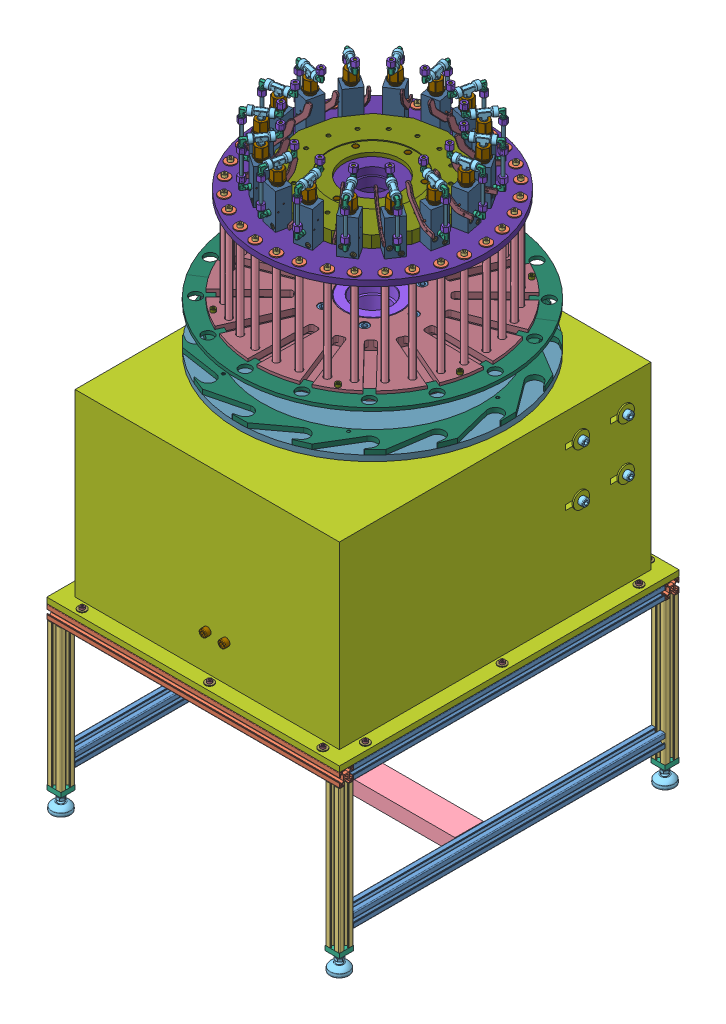
SolidWorks assembly Assieme_FINALE, configuration Default. Lengths in mm.
Overall size (1084.72 1264.83 1084.72).
659 component instances, 53 part files, 36 mates.
Components (placement in the parent):
- SupportoBase_Totale-2: SupportoBase_Totale [Default] at (4.0127 -14.4529 -3.9361) x (0 1 0) z (0 0 1) size (801.2 636.12 736.12)
  - Supporto_base_macchina-1: Supporto_base_macchina [Default] at origin size (378.2 636.12 736.12)
    - profilato_30x30_590-3: profilato_30x30_590 [Default] at (275.414 713.7262 -66.645) size (30 30 660)
    - profilato_30x30_590-5: profilato_30x30_590 [Default] at (275.414 123.7262 -66.645) size (30 30 660)
    - profilato_30x30_550-5: profilato_30x30_550 [Default] at (275.414 703.7262 -716.645) x (1 0 0) z (0 1 0) size (30 30 620)
    - profilato_30x30_550-6: profilato_30x30_550 [Default] at (275.414 703.7262 -26.645) x (1 0 0) z (0 1 0) size (30 30 620)
    - profilato_30x30_272-5: profilato_30x30_272 [Default] at (-16.586 123.7262 -716.645) x (0 0 1) z (-1 0 0) size (30 30 302)
    - profilato_30x30_272-6: profilato_30x30_272 [Default] at (-16.586 713.7262 -716.645) x (0 0 1) z (-1 0 0) size (30 30 302)
    - profilato_30x30_272-7: profilato_30x30_272 [Default] at (235.414 123.7262 -26.645) x (0 0 -1) z (1 0 0) size (30 30 302)
    - profilato_30x30_272-8: profilato_30x30_272 [Default] at (-16.586 713.7262 -26.645) x (0 0 1) z (-1 0 0) size (30 30 302)
    - profilo_U_60x30_490_supporto_base_macchina-1: profilo_U_60x30_490_supporto_base_macchina [Default] at (15.1 707.7262 -323.6583) x (0 0 1) z (0 -1 0) size (60 30 569)
    - profilato_30x30_590-6: profilato_30x30_590 [Default] at (3.414 123.7262 -66.645) size (30 30 660)
    - profilato_30x30_590-7: profilato_30x30_590 [Default] at (3.414 713.7262 -676.645) x (-1 0 0) z (0 0 -1) size (30 30 660)
    - 6322125-1: 6322125 [Default] at (-85.2818 713.7262 -26.645) x (0 0 -1) z (1 0 0) size (40 40 71.2)
    - 6322125-2: 6322125 [Default] at (-85.2818 713.7262 -716.645) x (0 0 -1) z (1 0 0) size (40 40 71.2)
    - 6322125-3: 6322125 [Default] at (-85.2818 123.7262 -26.645) x (0 -0.924225 -0.381849) z (1 0 0) size (40 40 71.2)
    - 6322125-4: 6322125 [Default] at (-85.2818 123.7262 -716.645) x (0 0 -1) z (1 0 0) size (40 40 71.2)
    - tappo_filettato_Supporto_base_macchina-1: tappo_filettato_Supporto_base_macchina [Default] at (-41.586 123.7262 -26.645) x (0 0 1) z (-1 0 0) size (30 30 10.37)
    - tappo_filettato_Supporto_base_macchina-2: tappo_filettato_Supporto_base_macchina [Default] at (-41.586 123.7262 -716.645) x (0 0 1) z (-1 0 0) size (30 30 10.37)
    - tappo_filettato_Supporto_base_macchina-3: tappo_filettato_Supporto_base_macchina [Default] at (-41.586 713.7262 -716.645) x (0 0 1) z (-1 0 0) size (30 30 10.37)
    - tappo_filettato_Supporto_base_macchina-4: tappo_filettato_Supporto_base_macchina [Default] at (-51.586 713.7262 -26.645) x (0 0 -1) z (1 0 0) size (30 30 10.37)
  - assieme_base-1: assieme_base [Default] at (466.8009 1138.7262 -472.0974) x (0 0 -1) z (0 -1 0) size (720 423 620)
    - Supporto di Base per macchina-1: Supporto di Base per macchina [Default] at (-460.4524 -176.3869 1030) size (720 403 620)
    - canotto di supporto-1: canotto di supporto [Default] at (-100.4524 134.8265 740) x (0 1 0) z (-0.866025 0 0.5) size (220 238 238)
    - m10 35mm-7: m10 35mm [ISO 4762 M10 x 35 - 35N] at (4.5476 246.6131 740) x (0 -1 0) z (1 0 0) size (45 16 16)
    - m10 35mm-8: m10 35mm [ISO 4762 M10 x 35 - 35N] at (-47.9524 246.6131 649.0673) x (0 -1 0) z (0.5 0 -0.866025) size (45 16 16)
    - m10 35mm-9: m10 35mm [ISO 4762 M10 x 35 - 35N] at (-152.9524 246.6131 649.0673) x (0 -1 0) z (-0.5 0 -0.866025) size (45 16 16)
    - m10 35mm-10: m10 35mm [ISO 4762 M10 x 35 - 35N] at (-205.4524 246.6131 740) x (0 -1 0) z (-1 0 0) size (45 16 16)
    - m10 35mm-11: m10 35mm [ISO 4762 M10 x 35 - 35N] at (-152.9524 246.6131 830.9327) x (0 -1 0) z (-0.5 0 0.866025) size (45 16 16)
    - m10 35mm-12: m10 35mm [ISO 4762 M10 x 35 - 35N] at (-47.9524 246.6131 830.9327) x (0 -1 0) z (0.5 0 0.866025) size (45 16 16)
    - Traversa di blocco albero-1: Traversa di blocco albero [Default] at (-100.4524 -86.3869 772.5) size (644 42 65)
    - m10 35mm-13: m10 35mm [ISO 4762 M10 x 35 - 35N] at (239.5476 -86.3869 760) x (-1 0 0) z (0 -1 0) size (45 16 16)
    - m10 35mm-16: m10 35mm [ISO 4762 M10 x 35 - 35N] at (239.5476 -86.3869 720) x (-1 0 0) z (0 -1 0) size (45 16 16)
    - m10 35mm-17: m10 35mm [ISO 4762 M10 x 35 - 35N] at (-440.4524 -86.3869 720) x (1 0 0) z (0 1 0) size (45 16 16)
    - m10 35mm-18: m10 35mm [ISO 4762 M10 x 35 - 35N] at (-440.4524 -86.3869 760) x (1 0 0) z (0 1 0) size (45 16 16)
  - DadoT-2: DadoT [Default] at (288.4104 668.7262 -716.645) x (0 0 -1) z (0 -1 0) size (16.5 6 8)
  - DadoT-9: DadoT [Default] at (288.4104 668.7262 -26.645) x (0 0 -1) z (0 -1 0) size (16.5 6 8)
  - DadoT-10: DadoT [Default] at (288.6104 713.7262 -661.645) x (0 1 0) z (0 0 -1) size (16.5 6 8)
  - DadoT-11: DadoT [Default] at (288.6104 713.7262 -371.645) x (0 1 0) z (0 0 -1) size (16.5 6 8)
  - DadoT-12: DadoT [Default] at (288.6104 713.7262 -81.645) x (0 1 0) z (0 0 -1) size (16.5 6 8)
  - DadoT-13: DadoT [Default] at (288.6104 123.7262 -661.645) x (0 1 0) z (0 0 -1) size (16.5 6 8)
  - DadoT-15: DadoT [Default] at (288.6104 123.7262 -371.645) x (0 1 0) z (0 0 -1) size (16.5 6 8)
  - DadoT-17: DadoT [Default] at (288.6104 123.7262 -81.645) x (0 1 0) z (0 0 -1) size (16.5 6 8)
  - RosettaM6-1: RosettaM6 [Washer ISO 7093 - 6] at (302.414 713.7262 -661.645) x (-1 0 0) z (0 0 1) size (1.6 18 18)
  - ViteM6-20-1: ViteM6-20 [ISO 4762 M6 x 20 - 20S] at (308.414 713.7262 -661.645) x (-1 0 0) z (0 0 1) size (26 10 10)
  - RosettaM6-2: RosettaM6 [Washer ISO 7093 - 6] at (302.414 668.7262 -716.645) x (-1 0 0) z (0 0 1) size (1.6 18 18)
  - ViteM6-20-2: ViteM6-20 [ISO 4762 M6 x 20 - 20S] at (308.414 668.7262 -716.645) x (-1 0 0) z (0 0 1) size (26 10 10)
  - RosettaM6-3: RosettaM6 [Washer ISO 7093 - 6] at (302.414 713.7262 -371.645) x (-1 0 0) z (0 0 1) size (1.6 18 18)
  - RosettaM6-4: RosettaM6 [Washer ISO 7093 - 6] at (302.414 713.7262 -81.645) x (-1 0 0) z (0 0 1) size (1.6 18 18)
  - ViteM6-20-3: ViteM6-20 [ISO 4762 M6 x 20 - 20S] at (308.414 713.7262 -371.645) x (-1 0 0) z (0 0 1) size (26 10 10)
  - ViteM6-20-4: ViteM6-20 [ISO 4762 M6 x 20 - 20S] at (308.414 713.7262 -81.645) x (-1 0 0) z (0 0 1) size (26 10 10)
  - RosettaM6-5: RosettaM6 [Washer ISO 7093 - 6] at (302.414 123.7262 -661.645) x (-1 0 0) z (0 0 1) size (1.6 18 18)
  - ViteM6-20-5: ViteM6-20 [ISO 4762 M6 x 20 - 20S] at (308.414 123.7262 -661.645) x (-1 0 0) z (0 0 1) size (26 10 10)
  - RosettaM6-6: RosettaM6 [Washer ISO 7093 - 6] at (302.414 123.7262 -371.645) x (-1 0 0) z (0 0 1) size (1.6 18 18)
  - RosettaM6-7: RosettaM6 [Washer ISO 7093 - 6] at (302.414 123.7262 -81.645) x (-1 0 0) z (0 0 1) size (1.6 18 18)
  - ViteM6-20-6: ViteM6-20 [ISO 4762 M6 x 20 - 20S] at (308.414 123.7262 -371.645) x (-1 0 0) z (0 0 1) size (26 10 10)
  - ViteM6-20-7: ViteM6-20 [ISO 4762 M6 x 20 - 20S] at (308.414 123.7262 -81.645) x (-1 0 0) z (0 0 1) size (26 10 10)
  - ViteM6-20-8: ViteM6-20 [ISO 4762 M6 x 20 - 20S] at (308.414 398.7262 -716.645) x (-1 0 0) z (0 0 1) size (26 10 10)
  - RosettaM6-8: RosettaM6 [Washer ISO 7093 - 6] at (302.414 398.7262 -716.645) x (-1 0 0) z (0 0 1) size (1.6 18 18)
  - DadoT-19: DadoT [Default] at (288.4104 398.7262 -716.645) x (0 0 -1) z (0 -1 0) size (16.5 6 8)
  - DadoT-20: DadoT [Default] at (288.4104 158.7262 -716.645) x (0 0 -1) z (0 -1 0) size (16.5 6 8)
  - RosettaM6-9: RosettaM6 [Washer ISO 7093 - 6] at (302.414 158.7262 -716.645) x (-1 0 0) z (0 0 1) size (1.6 18 18)
  - ViteM6-20-9: ViteM6-20 [ISO 4762 M6 x 20 - 20S] at (308.414 158.7262 -716.645) x (-1 0 0) z (0 0 1) size (26 10 10)
  - DadoT-21: DadoT [Default] at (288.4104 668.7262 -26.645) x (0 0 -1) z (0 -1 0) size (16.5 6 8)
  - RosettaM6-10: RosettaM6 [Washer ISO 7093 - 6] at (302.414 668.7262 -26.645) x (-1 0 0) z (0 0 1) size (1.6 18 18)
  - ViteM6-20-10: ViteM6-20 [ISO 4762 M6 x 20 - 20S] at (308.414 668.7262 -26.645) x (-1 0 0) z (0 0 1) size (26 10 10)
  - DadoT-22: DadoT [Default] at (288.4104 158.7262 -26.645) x (0 0 -1) z (0 -1 0) size (16.5 6 8)
  - RosettaM6-11: RosettaM6 [Washer ISO 7093 - 6] at (302.414 158.7262 -26.645) x (-1 0 0) z (0 0 1) size (1.6 18 18)
  - ViteM6-20-11: ViteM6-20 [ISO 4762 M6 x 20 - 20S] at (308.414 158.7262 -26.645) x (-1 0 0) z (0 0 1) size (26 10 10)
  - ViteM6-20-12: ViteM6-20 [ISO 4762 M6 x 20 - 20S] at (308.414 398.7262 -26.645) x (-1 0 0) z (0 0 1) size (26 10 10)
  - RosettaM6-12: RosettaM6 [Washer ISO 7093 - 6] at (302.414 398.7262 -26.645) x (-1 0 0) z (0 0 1) size (1.6 18 18)
  - DadoT-23: DadoT [Default] at (288.4104 398.7262 -26.645) x (0 0 -1) z (0 -1 0) size (16.5 6 8)
- motoriduttore-1: motoriduttore [Default] at (-164.7135 275.9611 -1179.5811) x (0 0 1) z (-1 0 0) size (200 160 175)
- Assieme_Riduttore-1: Assieme_Riduttore [Default] at (-346.4148 520.923 -401.8673) x (0 1 0) z (0.342115 0 -0.939658) size (226 168.82 169.04)
  - AlberoRiduttore-1: AlberoRiduttore [Default] at (-61.6906 7.4655 211) size (201 29 29)
  - linguetta_uni6604_b_8x7x50-1: linguetta_uni6604_b_8x7x50 [Default] at (-116.7419 7.4655 226) x (1 0 0) z (0 1 0) size (50 7 8)
  - linguetta_uni6604_b_8x7x35-1: linguetta_uni6604_b_8x7x35 [Default] at (-33.7419 7.4655 226.5) x (1 0 0) z (0 1 0) size (35 7 8)
  - linguetta_uni6604_b_8x7x35-2: linguetta_uni6604_b_8x7x35 [Default] at (41.2581 7.4655 226.5) x (1 0 0) z (0 1 0) size (35 7 8)
  - ASSIEME-LASS-90-VERS-B-O-25-3D.step-1: ASSIEME-LASS-90-VERS-B-O-25-3D.step [Default] at (-111.3519 -70.5563 279.3493) x (-1 0 0) z (0 0.707107 -0.707107) size (64.28 105 105)
  - Rondella di fermo-1: Rondella di fermo [Default] at (-122.7419 7.4655 211) x (0 0.707107 -0.707107) z (-1 0 0) size (36 36 3)
  - M8 25 mm-1: M8 25 mm [ISO 4762 M8 x 25 - 25N] at (92.2581 7.4655 211) x (-1 0 0) z (0 1 0) size (33 13 13)
  - M8 25 mm-2: M8 25 mm [ISO 4762 M8 x 25 - 25N] at (-133.7419 7.4655 211) x (1 0 0) z (0 -0.707107 0.707107) size (33 13 13)
  - M6 16mm-3: M6 16mm [ISO 4762 M6 x 16 - 16N] at (-44.8119 40.5589 196.8286) x (-1 0 0) z (0 0.935687 0.352831) size (22 10 10)
  - M6 16mm-14: M6 16mm [ISO 4762 M6 x 16 - 16N] at (-44.8119 11.7394 175.2546) x (-1 0 0) z (0 0.773404 -0.633913) size (22 10 10)
  - M6 16mm-15: M6 16mm [ISO 4762 M6 x 16 - 16N] at (-44.8119 -21.354 189.426) x (-1 0 0) z (0 -0.162283 -0.986744) size (22 10 10)
  - M6 16mm-16: M6 16mm [ISO 4762 M6 x 16 - 16N] at (-44.8119 -25.6279 225.1714) x (-1 0 0) z (0 -0.935687 -0.352831) size (22 10 10)
  - M6 16mm-17: M6 16mm [ISO 4762 M6 x 16 - 16N] at (-44.8119 3.1916 246.7454) x (-1 0 0) z (0 -0.773404 0.633913) size (22 10 10)
  - M6 16mm-18: M6 16mm [ISO 4762 M6 x 16 - 16N] at (-44.8119 36.285 232.574) x (-1 0 0) z (0 0.162283 0.986744) size (22 10 10)
  - Parte1^Assieme_Riduttore-1: Parte1^Assieme_Riduttore [Default] at origin (virtual)
  - ruota dentata m22-4: ruota dentata m22 [Chain wheel ISO - 22Z 10A-1 --22SA36.0N] at (-59.7419 7.4655 211) x (1 0 0) z (0 -0.599278 0.800541) size (8.93 120.13 121.23)
  - Rondella di fermo-2: Rondella di fermo [Default] at (84.2581 7.4655 211) x (0 0 1) z (-1 0 0) size (36 36 3)
- socket head cap screw_iso-1: socket head cap screw_iso [ISO 4762 M10 x 40 - 40N] at (-121.7135 603.4611 -555.5811) x (-1 0 0) z (0 -0.924225 -0.381849) size (50 16 16)
- socket head cap screw_iso-2: socket head cap screw_iso [ISO 4762 M10 x 40 - 40N] at (-121.7135 492.4611 -555.5811) x (-1 0 0) z (0 0 1) size (50 16 16)
- socket head cap screw_iso-3: socket head cap screw_iso [ISO 4762 M10 x 40 - 40N] at (-121.7135 603.4611 -650.5811) x (-1 0 0) z (0 0 1) size (50 16 16)
- socket head cap screw_iso-4: socket head cap screw_iso [ISO 4762 M10 x 40 - 40N] at (-121.7135 492.4611 -650.5811) x (-1 0 0) z (0 0 1) size (50 16 16)
- hex nut style 2 gradeab_iso-1: hex nut style 2 gradeab_iso [ISO - 4033 - M10 - W - N] at (-174.0135 603.4611 -650.5811) x (0 0 1) z (-1 0 0) size (16 18.48 9.3)
- hex nut style 2 gradeab_iso-2: hex nut style 2 gradeab_iso [ISO - 4033 - M10 - W - N] at (-174.0135 603.4611 -555.5811) x (0 0 1) z (-1 0 0) size (16 18.48 9.3)
- hex nut style 2 gradeab_iso-3: hex nut style 2 gradeab_iso [ISO - 4033 - M10 - W - N] at (-174.0135 492.4611 -650.5811) x (0 0 1) z (-1 0 0) size (16 18.48 9.3)
- hex nut style 2 gradeab_iso-4: hex nut style 2 gradeab_iso [ISO - 4033 - M10 - W - N] at (-174.0135 492.4611 -555.5811) x (0 0 1) z (-1 0 0) size (16 18.48 9.3)
- plain washer xlarge grade c_iso-1: plain washer xlarge grade c_iso [Washer ISO 7094 - 10] at (-134.7135 603.4611 -555.5811) x (-1 0 0) z (0 0.924225 0.381849) size (3 34 34)
- plain washer xlarge grade c_iso-2: plain washer xlarge grade c_iso [Washer ISO 7094 - 10] at (-134.7135 492.4611 -555.5811) x (-1 0 0) z (0 0 1) size (3 34 34)
- plain washer xlarge grade c_iso-3: plain washer xlarge grade c_iso [Washer ISO 7094 - 10] at (-134.7135 492.4611 -650.5811) x (-1 0 0) z (0 0 1) size (3 34 34)
- plain washer xlarge grade c_iso-4: plain washer xlarge grade c_iso [Washer ISO 7094 - 10] at (-134.7135 603.4611 -650.5811) x (-1 0 0) z (0 0 1) size (3 34 34)
- assieme parte rotante-1: assieme parte rotante [Default] at (-50.0904 623.9178 -607.5231) x (0 1 0) z (-0.804112 0 0.594478) size (749.63 778.63 778.63)
  - albero rotazione piatti-1: albero rotazione piatti [Default] at (60.413 18.3637 415) size (415 200 200)
  - seger 100mm-1: seger 100mm [KS 1336 E - 100] at (-146.4567 18.3637 415) x (0 0 -1) z (1 0 0) size (107.55 112.98 3)
  - SKF - 6020 - 20,DE,NC,20_68-1: SKF - 6020 - 20,DE,NC,20_68 [SKF - 6020 - 20,DE,NC,20_68] at (-131.4567 18.3637 415) x (1 0 0) z (0 -0.434476 -0.900684) size (24 150 150)
  - calettatore d95-1: calettatore d95 [Default] at (-178.8867 18.3637 415) size (39.5 135 135)
  - Chain wheel ISO - 50Z 10A-1-1: Chain wheel ISO - 50Z 10A-1 [Chain wheel ISO - 50Z 10A-1 --50SB120H25L95.0N] at (-164.8867 18.3637 415) size (25 262.06 262.51)
  - Disco supporto montaggio e Colonne-1: Disco supporto montaggio e Colonne [Default] at (204.0433 18.3637 415) x (0 -0.866025 -0.5) z (1 0 0) size (499.6 499.6 29)
  - SKF - 6020 - 20,DE,NC,20_68-2: SKF - 6020 - 20,DE,NC,20_68 [SKF - 6020 - 20,DE,NC,20_68] at (62.0433 18.3637 415) x (1 0 0) z (0 -0.432628 -0.901573) size (24 150 150)
  - piatto rotante porta tappi-1: piatto rotante porta tappi [Default] at (99.0433 18.3637 415) x (0 0 -1) z (1 0 0) size (570 570 20.57)
  - disco trasportatore tappi 31-1: disco trasportatore tappi 31 [Default] at (111.0433 18.3637 415) x (0 0.5 -0.866025) z (1 0 0) size (570 570 10.42)
  - Distributore Rotante-1: Distributore Rotante [Default] at (425.0433 18.3637 415) x (0 -0.055301 -0.99847) z (1 0 0) size (310 310 25.54)
  - disco trascinato porta distributore vuoto-1: disco trascinato porta distributore vuoto [Default] at (400.0433 18.3637 415) x (0 0.055301 0.99847) z (-1 0 0) size (480 480 50)
  - m12 35mm-1: m12 35mm [ISO 4762 M12 x 35 - 35N] at (376.0433 -53.0243 378.8925) x (1 0 0) z (0 -0.5 0.866025) size (47 18 18)
  - m12 90mm-3: m12 90mm [ISO 4762 M12 x 90 - 90N] at (203.0433 -21.6363 345.718) x (-1 0 0) z (0 -0.5 0.866025) size (102 18 18)
  - rondella m6 22mm-1: rondella m6 22mm [Washer ISO 7094 - 6] at (99.0433 -101.6363 207.1539) x (1 0 0) z (0 -1 0) size (2 22 22)
  - M6 20mm-1: M6 20mm [ISO 4762 M6 x 20 - 20N] at (91.0433 -101.6363 207.1539) x (1 0 0) z (0 0.5 0.866025) size (26 10 10)
  - m12 35mm-2: m12 35mm [ISO 4762 M12 x 35 - 35N] at (376.0433 13.9397 335.1224) x (1 0 0) z (0 -1 0) size (47 18 18)
  - m12 35mm-3: m12 35mm [ISO 4762 M12 x 35 - 35N] at (376.0433 85.3277 371.2299) x (1 0 0) z (0 -0.5 -0.866025) size (47 18 18)
  - m12 35mm-4: m12 35mm [ISO 4762 M12 x 35 - 35N] at (376.0433 89.7517 451.1075) x (1 0 0) z (0 0.5 -0.866025) size (47 18 18)
  - m12 35mm-5: m12 35mm [ISO 4762 M12 x 35 - 35N] at (376.0433 22.7877 494.8776) x (1 0 0) z (0 1 0) size (47 18 18)
  - m12 35mm-6: m12 35mm [ISO 4762 M12 x 35 - 35N] at (376.0433 -48.6003 458.7701) x (1 0 0) z (0 0.5 0.866025) size (47 18 18)
  - rondella m6 22mm-2: rondella m6 22mm [Washer ISO 7094 - 6] at (99.0433 138.3637 207.1539) x (1 0 0) z (0 -0.5 -0.866025) size (2 22 22)
  - rondella m6 22mm-3: rondella m6 22mm [Washer ISO 7094 - 6] at (99.0433 258.3637 415) x (1 0 0) z (0 0.5 -0.866025) size (2 22 22)
  - rondella m6 22mm-4: rondella m6 22mm [Washer ISO 7094 - 6] at (99.0433 138.3637 622.8461) x (1 0 0) z (0 1 0) size (2 22 22)
  - rondella m6 22mm-5: rondella m6 22mm [Washer ISO 7094 - 6] at (99.0433 -101.6363 622.8461) x (1 0 0) z (0 0.5 0.866025) size (2 22 22)
  - rondella m6 22mm-6: rondella m6 22mm [Washer ISO 7094 - 6] at (99.0433 -221.6363 415) x (1 0 0) z (0 -0.5 0.866025) size (2 22 22)
  - M6 20mm-2: M6 20mm [ISO 4762 M6 x 20 - 20N] at (91.0433 138.3637 207.1539) x (1 0 0) z (0 -0.5 0.866025) size (26 10 10)
  - M6 20mm-3: M6 20mm [ISO 4762 M6 x 20 - 20N] at (91.0433 258.3637 415) x (1 0 0) z (0 -1 0) size (26 10 10)
  - M6 20mm-4: M6 20mm [ISO 4762 M6 x 20 - 20N] at (91.0433 138.3637 622.8461) x (1 0 0) z (0 -0.5 -0.866025) size (26 10 10)
  - M6 20mm-5: M6 20mm [ISO 4762 M6 x 20 - 20N] at (91.0433 -101.6363 622.8461) x (1 0 0) z (0 0.5 -0.866025) size (26 10 10)
  - M6 20mm-6: M6 20mm [ISO 4762 M6 x 20 - 20N] at (91.0433 -221.6363 415) x (1 0 0) z (0 1 0) size (26 10 10)
  - m12 90mm-4: m12 90mm [ISO 4762 M12 x 90 - 90N] at (203.0433 58.3637 345.718) x (-1 0 0) z (0 -1 0) size (102 18 18)
  - m12 90mm-5: m12 90mm [ISO 4762 M12 x 90 - 90N] at (203.0433 98.3637 415) x (-1 0 0) z (0 -0.5 -0.866025) size (102 18 18)
  - m12 90mm-6: m12 90mm [ISO 4762 M12 x 90 - 90N] at (203.0433 58.3637 484.282) x (-1 0 0) z (0 0.5 -0.866025) size (102 18 18)
  - m12 90mm-7: m12 90mm [ISO 4762 M12 x 90 - 90N] at (203.0433 -21.6363 484.282) x (-1 0 0) z (0 1 0) size (102 18 18)
  - m12 90mm-8: m12 90mm [ISO 4762 M12 x 90 - 90N] at (203.0433 -61.6363 415) x (-1 0 0) z (0 0.5 0.866025) size (102 18 18)
  - asta scorrimento carello-1: asta scorrimento carello [Default] at (287.5433 70.1437 197.9013) x (0 0 -1) z (1 0 0) size (12 12 225)
  - rondella m6 22mm-7: rondella m6 22mm [Washer ISO 7094 - 6] at (175.0433 70.1437 197.9013) x (1 0 0) z (0 -1 0) size (2 22 22)
  - M6 16mm-1: M6 16mm [ISO 4762 M6 x 16 - 16N] at (167.0433 70.1437 197.9013) size (22 10 10)
  - M6 16mm-2: M6 16mm [ISO 4762 M6 x 16 - 16N] at (408.0433 70.1437 197.9013) x (-1 0 0) z (0 0 -1) size (22 10 10)
  - rondella m6 22mm-8: rondella m6 22mm [Washer ISO 7094 - 6] at (400.0433 70.1437 197.9013) x (-1 0 0) z (0 1 0) size (2 22 22)
  - rondella m6 22mm-9: rondella m6 22mm [Washer ISO 7094 - 6] at (175.0433 24.5373 191.8971) x (1 0 0) z (0 -0.965926 -0.258819) size (2 22 22)
  - M6 16mm-3: M6 16mm [ISO 4762 M6 x 16 - 16N] at (167.0433 24.5373 191.8971) x (1 0 0) z (0 0.258819 -0.965926) size (22 10 10)
  - asta scorrimento carello-2: asta scorrimento carello [Default] at (287.5433 24.5373 191.8971) x (0 0.258819 -0.965926) z (-1 0 0) size (12 12 225)
  - rondella m6 22mm-10: rondella m6 22mm [Washer ISO 7094 - 6] at (400.0433 24.5373 191.8971) x (-1 0 0) z (0 0.965926 0.258819) size (2 22 22)
  - M6 16mm-4: M6 16mm [ISO 4762 M6 x 16 - 16N] at (408.0433 24.5373 191.8971) x (-1 0 0) z (0 -0.258819 0.965926) size (22 10 10)
  - AssiemeValvola-1: AssiemeValvola [Default] at (515.3257 74.6348 254.5832) x (0 -0.331007 0.943628) z (0 0.943628 0.331007) size (90.26 138.63 38)
    - RaccordoT-1: RaccordoT [Default] at origin size (43 29.75 16.5)
    - Raccordo a L-1: Raccordo a L [Default] at (-30 0 0) x (0 -1 0) z (0 0 -1) size (28.34 25.51 14.01)
      - 1809_06_10_01-1: 1809_06_10_01 [Default] at origin size (22.49 23 10)
      - 1809_06_10_02-1: 1809_06_10_02 [Default] at origin size (6.5 8.5 8.5)
      - 1809_06_10_03-1: 1809_06_10_03 [Default] at origin size (11.02 15.01 14.01)
    - Raccordo a L-2: Raccordo a L [Default] at (30 0 0) x (0 1 0) z (0 0 -1) size (28.34 25.51 14.01)
      - 1809_06_10_01-1: 1809_06_10_01 [Default] at origin size (22.49 23 10)
      - 1809_06_10_02-1: 1809_06_10_02 [Default] at origin size (6.5 8.5 8.5)
      - 1809_06_10_03-1: 1809_06_10_03 [Default] at origin size (11.02 15.01 14.01)
    - TappoChiusura-1: TappoChiusura [Default] at (0 -32 0) x (0 -1 0) z (0 0 1) size (38.28 26.74 26.74)
    - CorpoValvola-1: CorpoValvola [Default] at (-15 -115.2824 0) size (30 75 34)
    - Raccordo a L-3: Raccordo a L [Default] at (-30 -88.2824 0) x (0 1 0) z (0 0 1) size (28.34 25.51 14.01)
      - 1809_06_10_01-1: 1809_06_10_01 [Default] at origin size (22.49 23 10)
      - 1809_06_10_02-1: 1809_06_10_02 [Default] at origin size (6.5 8.5 8.5)
      - 1809_06_10_03-1: 1809_06_10_03 [Default] at origin size (11.02 15.01 14.01)
    - Spina_3x38-1: Spina_3x38 [Default] at (0 -68.2824 -21) x (-1 0 0) z (0 0 1) size (3 3 38)
    - Spina_3x38-2: Spina_3x38 [Default] at (-10 -80.2824 -21) x (0.996193 0.087174 0) z (0 0 1) size (3 3 38)
    - M5 40mm-3: M5 40mm [ISO 4762 M5 x 40 - 40N] at (-14.6 -108.7824 9) size (45 8.5 8.5)
    - M5 40mm-2: M5 40mm [ISO 4762 M5 x 40 - 40N] at (-14.6 -96.7824 -9) size (45 8.5 8.5)
    - LevaValvola-1: LevaValvola [Default] at (-24.507 -86.571 -17) x (0.996193 0.087174 0) z (0 0 1) size (77.55 60.2 4)
    - Tubo-1: Tubo [Default] at (-30 -15.9665 0) x (1 0 0) z (0 -1 0) size (6 6 56.4)
  - M6 16mm-5: M6 16mm [ISO 4762 M6 x 16 - 16N] at (167.0433 -16.8778 194.6116) x (1 0 0) z (0 0.382683 0.92388) size (22 10 10)
  - M6 16mm-6: M6 16mm [ISO 4762 M6 x 16 - 16N] at (167.0433 -98.5342 224.874) x (1 0 0) z (0 0.707107 0.707107) size (22 10 10)
  - M6 16mm-7: M6 16mm [ISO 4762 M6 x 16 - 16N] at (167.0433 -162.3939 284.0814) x (1 0 0) z (0 0.92388 0.382683) size (22 10 10)
  - M6 16mm-8: M6 16mm [ISO 4762 M6 x 16 - 16N] at (167.0433 -198.735 363.22) x (1 0 0) z (0 1 0) size (22 10 10)
  - M6 16mm-9: M6 16mm [ISO 4762 M6 x 16 - 16N] at (167.0433 -202.0247 450.2415) x (1 0 0) z (0 0.92388 -0.382683) size (22 10 10)
  - M6 16mm-10: M6 16mm [ISO 4762 M6 x 16 - 16N] at (167.0433 -171.7623 531.8979) x (1 0 0) z (0 0.707107 -0.707107) size (22 10 10)
  - M6 16mm-11: M6 16mm [ISO 4762 M6 x 16 - 16N] at (167.0433 -112.5549 595.7576) x (1 0 0) z (0 0.382683 -0.92388) size (22 10 10)
  - M6 16mm-12: M6 16mm [ISO 4762 M6 x 16 - 16N] at (167.0433 -33.4163 632.0987) x (1 0 0) z (0 0 -1) size (22 10 10)
  - M6 16mm-13: M6 16mm [ISO 4762 M6 x 16 - 16N] at (167.0433 53.6052 635.3884) x (1 0 0) z (0 -0.382683 -0.92388) size (22 10 10)
  - M6 16mm-14: M6 16mm [ISO 4762 M6 x 16 - 16N] at (167.0433 135.2616 605.126) x (1 0 0) z (0 -0.707107 -0.707107) size (22 10 10)
  - M6 16mm-15: M6 16mm [ISO 4762 M6 x 16 - 16N] at (167.0433 199.1213 545.9186) x (1 0 0) z (0 -0.92388 -0.382683) size (22 10 10)
  - M6 16mm-16: M6 16mm [ISO 4762 M6 x 16 - 16N] at (167.0433 235.4624 466.78) x (1 0 0) z (0 -1 0) size (22 10 10)
  - M6 16mm-17: M6 16mm [ISO 4762 M6 x 16 - 16N] at (167.0433 238.7521 379.7585) x (1 0 0) z (0 -0.92388 0.382683) size (22 10 10)
  - M6 16mm-18: M6 16mm [ISO 4762 M6 x 16 - 16N] at (167.0433 208.4897 298.1021) x (1 0 0) z (0 -0.707107 0.707107) size (22 10 10)
  - M6 16mm-19: M6 16mm [ISO 4762 M6 x 16 - 16N] at (167.0433 149.2823 234.2424) x (1 0 0) z (0 -0.382683 0.92388) size (22 10 10)
  - rondella m6 22mm-11: rondella m6 22mm [Washer ISO 7094 - 6] at (175.0433 -16.8778 194.6116) x (1 0 0) z (0 -0.92388 0.382683) size (2 22 22)
  - rondella m6 22mm-12: rondella m6 22mm [Washer ISO 7094 - 6] at (175.0433 -98.5342 224.874) x (1 0 0) z (0 -0.707107 0.707107) size (2 22 22)
  - rondella m6 22mm-13: rondella m6 22mm [Washer ISO 7094 - 6] at (175.0433 -162.3939 284.0814) x (1 0 0) z (0 -0.382683 0.92388) size (2 22 22)
  - rondella m6 22mm-14: rondella m6 22mm [Washer ISO 7094 - 6] at (175.0433 -198.735 363.22) size (2 22 22)
  - rondella m6 22mm-15: rondella m6 22mm [Washer ISO 7094 - 6] at (175.0433 -202.0247 450.2415) x (1 0 0) z (0 0.382683 0.92388) size (2 22 22)
  - rondella m6 22mm-16: rondella m6 22mm [Washer ISO 7094 - 6] at (175.0433 -171.7623 531.8979) x (1 0 0) z (0 0.707107 0.707107) size (2 22 22)
  - rondella m6 22mm-17: rondella m6 22mm [Washer ISO 7094 - 6] at (175.0433 -112.5549 595.7576) x (1 0 0) z (0 0.92388 0.382683) size (2 22 22)
  - rondella m6 22mm-18: rondella m6 22mm [Washer ISO 7094 - 6] at (175.0433 -33.4163 632.0987) x (1 0 0) z (0 1 0) size (2 22 22)
  - rondella m6 22mm-19: rondella m6 22mm [Washer ISO 7094 - 6] at (175.0433 53.6052 635.3884) x (1 0 0) z (0 0.92388 -0.382683) size (2 22 22)
  - rondella m6 22mm-20: rondella m6 22mm [Washer ISO 7094 - 6] at (175.0433 135.2616 605.126) x (1 0 0) z (0 0.707107 -0.707107) size (2 22 22)
  - rondella m6 22mm-21: rondella m6 22mm [Washer ISO 7094 - 6] at (175.0433 199.1213 545.9186) x (1 0 0) z (0 0.382683 -0.92388) size (2 22 22)
  - rondella m6 22mm-22: rondella m6 22mm [Washer ISO 7094 - 6] at (175.0433 235.4624 466.78) x (1 0 0) z (0 0 -1) size (2 22 22)
  - rondella m6 22mm-23: rondella m6 22mm [Washer ISO 7094 - 6] at (175.0433 238.7521 379.7585) x (1 0 0) z (0 -0.382683 -0.92388) size (2 22 22)
  - rondella m6 22mm-24: rondella m6 22mm [Washer ISO 7094 - 6] at (175.0433 208.4897 298.1021) x (1 0 0) z (0 -0.707107 -0.707107) size (2 22 22)
  - rondella m6 22mm-25: rondella m6 22mm [Washer ISO 7094 - 6] at (175.0433 149.2823 234.2424) x (1 0 0) z (0 -0.92388 -0.382683) size (2 22 22)
  - asta scorrimento carello-3: asta scorrimento carello [Default] at (287.5433 -16.8778 194.6116) x (0 -0.382683 -0.92388) z (1 0 0) size (12 12 225)
  - asta scorrimento carello-4: asta scorrimento carello [Default] at (287.5433 -98.5342 224.874) x (0 -0.707107 -0.707107) z (1 0 0) size (12 12 225)
  - asta scorrimento carello-5: asta scorrimento carello [Default] at (287.5433 -162.3939 284.0814) x (0 -0.92388 -0.382683) z (1 0 0) size (12 12 225)
  - asta scorrimento carello-6: asta scorrimento carello [Default] at (287.5433 -198.735 363.22) x (0 -1 0) z (1 0 0) size (12 12 225)
  - asta scorrimento carello-7: asta scorrimento carello [Default] at (287.5433 -202.0247 450.2415) x (0 -0.92388 0.382683) z (1 0 0) size (12 12 225)
  - asta scorrimento carello-8: asta scorrimento carello [Default] at (287.5433 -171.7623 531.8979) x (0 -0.707107 0.707107) z (1 0 0) size (12 12 225)
  - asta scorrimento carello-9: asta scorrimento carello [Default] at (287.5433 -112.5549 595.7576) x (0 -0.382683 0.92388) z (1 0 0) size (12 12 225)
  - asta scorrimento carello-10: asta scorrimento carello [Default] at (287.5433 -33.4163 632.0987) x (0 0 1) z (1 0 0) size (12 12 225)
  - asta scorrimento carello-11: asta scorrimento carello [Default] at (287.5433 53.6052 635.3884) x (0 0.382683 0.92388) z (1 0 0) size (12 12 225)
  - asta scorrimento carello-12: asta scorrimento carello [Default] at (287.5433 135.2616 605.126) x (0 0.707107 0.707107) z (1 0 0) size (12 12 225)
  - asta scorrimento carello-13: asta scorrimento carello [Default] at (287.5433 199.1213 545.9186) x (0 0.92388 0.382683) z (1 0 0) size (12 12 225)
  - asta scorrimento carello-14: asta scorrimento carello [Default] at (287.5433 235.4624 466.78) x (0 1 0) z (1 0 0) size (12 12 225)
  - asta scorrimento carello-15: asta scorrimento carello [Default] at (287.5433 238.7521 379.7585) x (0 0.92388 -0.382683) z (1 0 0) size (12 12 225)
  - asta scorrimento carello-16: asta scorrimento carello [Default] at (287.5433 208.4897 298.1021) x (0 0.707107 -0.707107) z (1 0 0) size (12 12 225)
  - asta scorrimento carello-17: asta scorrimento carello [Default] at (287.5433 149.2823 234.2424) x (0 0.382683 -0.92388) z (1 0 0) size (12 12 225)
  - M6 16mm-20: M6 16mm [ISO 4762 M6 x 16 - 16N] at (408.0433 -16.8778 194.6116) x (-1 0 0) z (0 -0.382683 -0.92388) size (22 10 10)
  - M6 16mm-21: M6 16mm [ISO 4762 M6 x 16 - 16N] at (408.0433 -98.5342 224.874) x (-1 0 0) z (0 -0.707107 -0.707107) size (22 10 10)
  - M6 16mm-22: M6 16mm [ISO 4762 M6 x 16 - 16N] at (408.0433 -162.3939 284.0814) x (-1 0 0) z (0 -0.92388 -0.382683) size (22 10 10)
  - M6 16mm-23: M6 16mm [ISO 4762 M6 x 16 - 16N] at (408.0433 -198.735 363.22) x (-1 0 0) z (0 -1 0) size (22 10 10)
  - M6 16mm-24: M6 16mm [ISO 4762 M6 x 16 - 16N] at (408.0433 -202.0247 450.2415) x (-1 0 0) z (0 -0.92388 0.382683) size (22 10 10)
  - M6 16mm-25: M6 16mm [ISO 4762 M6 x 16 - 16N] at (408.0433 -171.7623 531.8979) x (-1 0 0) z (0 -0.707107 0.707107) size (22 10 10)
  - M6 16mm-26: M6 16mm [ISO 4762 M6 x 16 - 16N] at (408.0433 -112.5549 595.7576) x (-1 0 0) z (0 -0.382683 0.92388) size (22 10 10)
  - M6 16mm-27: M6 16mm [ISO 4762 M6 x 16 - 16N] at (408.0433 -33.4163 632.0987) x (-1 0 0) z (0 0 1) size (22 10 10)
  - M6 16mm-28: M6 16mm [ISO 4762 M6 x 16 - 16N] at (408.0433 53.6052 635.3884) x (-1 0 0) z (0 0.382683 0.92388) size (22 10 10)
  - M6 16mm-29: M6 16mm [ISO 4762 M6 x 16 - 16N] at (408.0433 135.2616 605.126) x (-1 0 0) z (0 0.707107 0.707107) size (22 10 10)
  - M6 16mm-30: M6 16mm [ISO 4762 M6 x 16 - 16N] at (408.0433 199.1213 545.9186) x (-1 0 0) z (0 0.92388 0.382683) size (22 10 10)
  - M6 16mm-31: M6 16mm [ISO 4762 M6 x 16 - 16N] at (408.0433 235.4624 466.78) x (-1 0 0) z (0 1 0) size (22 10 10)
  - M6 16mm-32: M6 16mm [ISO 4762 M6 x 16 - 16N] at (408.0433 238.7521 379.7585) x (-1 0 0) z (0 0.92388 -0.382683) size (22 10 10)
  - M6 16mm-33: M6 16mm [ISO 4762 M6 x 16 - 16N] at (408.0433 208.4897 298.1021) x (-1 0 0) z (0 0.707107 -0.707107) size (22 10 10)
  - M6 16mm-34: M6 16mm [ISO 4762 M6 x 16 - 16N] at (408.0433 149.2823 234.2424) x (-1 0 0) z (0 0.382683 -0.92388) size (22 10 10)
  - rondella m6 22mm-26: rondella m6 22mm [Washer ISO 7094 - 6] at (400.0433 -16.8778 194.6116) x (-1 0 0) z (0 0.92388 -0.382683) size (2 22 22)
  - rondella m6 22mm-27: rondella m6 22mm [Washer ISO 7094 - 6] at (400.0433 -98.5342 224.874) x (-1 0 0) z (0 0.707107 -0.707107) size (2 22 22)
  - rondella m6 22mm-28: rondella m6 22mm [Washer ISO 7094 - 6] at (400.0433 -162.3939 284.0814) x (-1 0 0) z (0 0.382683 -0.92388) size (2 22 22)
  - rondella m6 22mm-29: rondella m6 22mm [Washer ISO 7094 - 6] at (400.0433 -198.735 363.22) x (-1 0 0) z (0 0 -1) size (2 22 22)
  - rondella m6 22mm-30: rondella m6 22mm [Washer ISO 7094 - 6] at (400.0433 -202.0247 450.2415) x (-1 0 0) z (0 -0.382683 -0.92388) size (2 22 22)
  - rondella m6 22mm-31: rondella m6 22mm [Washer ISO 7094 - 6] at (400.0433 -171.7623 531.8979) x (-1 0 0) z (0 -0.707107 -0.707107) size (2 22 22)
  - rondella m6 22mm-32: rondella m6 22mm [Washer ISO 7094 - 6] at (400.0433 -112.5549 595.7576) x (-1 0 0) z (0 -0.92388 -0.382683) size (2 22 22)
  - rondella m6 22mm-33: rondella m6 22mm [Washer ISO 7094 - 6] at (400.0433 -33.4163 632.0987) x (-1 0 0) z (0 -1 0) size (2 22 22)
  - rondella m6 22mm-34: rondella m6 22mm [Washer ISO 7094 - 6] at (400.0433 53.6052 635.3884) x (-1 0 0) z (0 -0.92388 0.382683) size (2 22 22)
  - rondella m6 22mm-35: rondella m6 22mm [Washer ISO 7094 - 6] at (400.0433 135.2616 605.126) x (-1 0 0) z (0 -0.707107 0.707107) size (2 22 22)
  - rondella m6 22mm-36: rondella m6 22mm [Washer ISO 7094 - 6] at (400.0433 199.1213 545.9186) x (-1 0 0) z (0 -0.382683 0.92388) size (2 22 22)
  - rondella m6 22mm-37: rondella m6 22mm [Washer ISO 7094 - 6] at (400.0433 235.4624 466.78) x (-1 0 0) z (0 0 1) size (2 22 22)
  - rondella m6 22mm-38: rondella m6 22mm [Washer ISO 7094 - 6] at (400.0433 238.7521 379.7585) x (-1 0 0) z (0 0.382683 0.92388) size (2 22 22)
  - rondella m6 22mm-39: rondella m6 22mm [Washer ISO 7094 - 6] at (400.0433 208.4897 298.1021) x (-1 0 0) z (0 0.707107 0.707107) size (2 22 22)
  - rondella m6 22mm-40: rondella m6 22mm [Washer ISO 7094 - 6] at (400.0433 149.2823 234.2424) x (-1 0 0) z (0 0.92388 0.382683) size (2 22 22)
  - rondella m6 22mm-41: rondella m6 22mm [Washer ISO 7094 - 6] at (175.0433 -61.3104 206.5173) x (1 0 0) z (0 -0.991445 0.130526) size (2 22 22)
  - rondella m6 22mm-42: rondella m6 22mm [Washer ISO 7094 - 6] at (175.0433 -135.0285 252.8771) x (1 0 0) z (0 -0.866025 0.5) size (2 22 22)
  - rondella m6 22mm-43: rondella m6 22mm [Washer ISO 7094 - 6] at (175.0433 -185.3939 323.9186) x (1 0 0) z (0 -0.608761 0.793353) size (2 22 22)
  - rondella m6 22mm-44: rondella m6 22mm [Washer ISO 7094 - 6] at (175.0433 -204.7392 408.8264) x (1 0 0) z (0 -0.258819 0.965926) size (2 22 22)
  - rondella m6 22mm-45: rondella m6 22mm [Washer ISO 7094 - 6] at (175.0433 -190.119 494.6741) x (1 0 0) z (0 0.130526 0.991445) size (2 22 22)
  - rondella m6 22mm-46: rondella m6 22mm [Washer ISO 7094 - 6] at (175.0433 -143.7592 568.3922) x (1 0 0) z (0 0.5 0.866025) size (2 22 22)
  - rondella m6 22mm-47: rondella m6 22mm [Washer ISO 7094 - 6] at (175.0433 -72.7177 618.7576) x (1 0 0) z (0 0.793353 0.608761) size (2 22 22)
  - rondella m6 22mm-48: rondella m6 22mm [Washer ISO 7094 - 6] at (175.0433 12.1901 638.1029) x (1 0 0) z (0 0.965926 0.258819) size (2 22 22)
  - rondella m6 22mm-49: rondella m6 22mm [Washer ISO 7094 - 6] at (175.0433 98.0378 623.4827) x (1 0 0) z (0 0.991445 -0.130526) size (2 22 22)
  - rondella m6 22mm-50: rondella m6 22mm [Washer ISO 7094 - 6] at (175.0433 171.7559 577.1229) x (1 0 0) z (0 0.866025 -0.5) size (2 22 22)
  - rondella m6 22mm-51: rondella m6 22mm [Washer ISO 7094 - 6] at (175.0433 222.1213 506.0814) x (1 0 0) z (0 0.608761 -0.793353) size (2 22 22)
  - rondella m6 22mm-52: rondella m6 22mm [Washer ISO 7094 - 6] at (175.0433 241.4666 421.1736) x (1 0 0) z (0 0.258819 -0.965926) size (2 22 22)
  - rondella m6 22mm-53: rondella m6 22mm [Washer ISO 7094 - 6] at (175.0433 226.8464 335.3259) x (1 0 0) z (0 -0.130526 -0.991445) size (2 22 22)
  - rondella m6 22mm-54: rondella m6 22mm [Washer ISO 7094 - 6] at (175.0433 180.4866 261.6078) x (1 0 0) z (0 -0.5 -0.866025) size (2 22 22)
  - rondella m6 22mm-55: rondella m6 22mm [Washer ISO 7094 - 6] at (175.0433 109.4451 211.2424) x (1 0 0) z (0 -0.793353 -0.608761) size (2 22 22)
  - M6 16mm-35: M6 16mm [ISO 4762 M6 x 16 - 16N] at (167.0433 -61.3104 206.5173) x (1 0 0) z (0 -0.130526 -0.991445) size (22 10 10)
  - M6 16mm-36: M6 16mm [ISO 4762 M6 x 16 - 16N] at (167.0433 -135.0285 252.8771) x (1 0 0) z (0 -0.5 -0.866025) size (22 10 10)
  - M6 16mm-37: M6 16mm [ISO 4762 M6 x 16 - 16N] at (167.0433 -185.3939 323.9186) x (1 0 0) z (0 -0.793353 -0.608761) size (22 10 10)
  - M6 16mm-38: M6 16mm [ISO 4762 M6 x 16 - 16N] at (167.0433 -204.7392 408.8264) x (1 0 0) z (0 -0.965926 -0.258819) size (22 10 10)
  - M6 16mm-39: M6 16mm [ISO 4762 M6 x 16 - 16N] at (167.0433 -190.119 494.6741) x (1 0 0) z (0 -0.991445 0.130526) size (22 10 10)
  - M6 16mm-40: M6 16mm [ISO 4762 M6 x 16 - 16N] at (167.0433 -143.7592 568.3922) x (1 0 0) z (0 -0.866025 0.5) size (22 10 10)
  - M6 16mm-41: M6 16mm [ISO 4762 M6 x 16 - 16N] at (167.0433 -72.7177 618.7576) x (1 0 0) z (0 -0.608761 0.793353) size (22 10 10)
  - M6 16mm-42: M6 16mm [ISO 4762 M6 x 16 - 16N] at (167.0433 12.1901 638.1029) x (1 0 0) z (0 -0.258819 0.965926) size (22 10 10)
  - M6 16mm-43: M6 16mm [ISO 4762 M6 x 16 - 16N] at (167.0433 98.0378 623.4827) x (1 0 0) z (0 0.130526 0.991445) size (22 10 10)
  - M6 16mm-44: M6 16mm [ISO 4762 M6 x 16 - 16N] at (167.0433 171.7559 577.1229) x (1 0 0) z (0 0.5 0.866025) size (22 10 10)
  - M6 16mm-45: M6 16mm [ISO 4762 M6 x 16 - 16N] at (167.0433 222.1213 506.0814) x (1 0 0) z (0 0.793353 0.608761) size (22 10 10)
  - M6 16mm-46: M6 16mm [ISO 4762 M6 x 16 - 16N] at (167.0433 241.4666 421.1736) x (1 0 0) z (0 0.965926 0.258819) size (22 10 10)
  - M6 16mm-47: M6 16mm [ISO 4762 M6 x 16 - 16N] at (167.0433 226.8464 335.3259) x (1 0 0) z (0 0.991445 -0.130526) size (22 10 10)
  - M6 16mm-48: M6 16mm [ISO 4762 M6 x 16 - 16N] at (167.0433 180.4866 261.6078) x (1 0 0) z (0 0.866025 -0.5) size (22 10 10)
  - M6 16mm-49: M6 16mm [ISO 4762 M6 x 16 - 16N] at (167.0433 109.4451 211.2424) x (1 0 0) z (0 0.608761 -0.793353) size (22 10 10)
  - asta scorrimento carello-18: asta scorrimento carello [Default] at (287.5433 -61.3104 206.5173) x (0 -0.130526 -0.991445) z (-1 0 0) size (12 12 225)
  - asta scorrimento carello-19: asta scorrimento carello [Default] at (287.5433 -135.0285 252.8771) x (0 -0.5 -0.866025) z (-1 0 0) size (12 12 225)
  - asta scorrimento carello-20: asta scorrimento carello [Default] at (287.5433 -185.3939 323.9186) x (0 -0.793353 -0.608761) z (-1 0 0) size (12 12 225)
  - asta scorrimento carello-21: asta scorrimento carello [Default] at (287.5433 -204.7392 408.8264) x (0 -0.965926 -0.258819) z (-1 0 0) size (12 12 225)
  - asta scorrimento carello-22: asta scorrimento carello [Default] at (287.5433 -190.119 494.6741) x (0 -0.991445 0.130526) z (-1 0 0) size (12 12 225)
  - asta scorrimento carello-23: asta scorrimento carello [Default] at (287.5433 -143.7592 568.3922) x (0 -0.866025 0.5) z (-1 0 0) size (12 12 225)
  - asta scorrimento carello-24: asta scorrimento carello [Default] at (287.5433 -72.7177 618.7576) x (0 -0.608761 0.793353) z (-1 0 0) size (12 12 225)
  - asta scorrimento carello-25: asta scorrimento carello [Default] at (287.5433 12.1901 638.1029) x (0 -0.258819 0.965926) z (-1 0 0) size (12 12 225)
  - asta scorrimento carello-26: asta scorrimento carello [Default] at (287.5433 98.0378 623.4827) x (0 0.130526 0.991445) z (-1 0 0) size (12 12 225)
  - asta scorrimento carello-27: asta scorrimento carello [Default] at (287.5433 171.7559 577.1229) x (0 0.5 0.866025) z (-1 0 0) size (12 12 225)
  - asta scorrimento carello-28: asta scorrimento carello [Default] at (287.5433 222.1213 506.0814) x (0 0.793353 0.608761) z (-1 0 0) size (12 12 225)
  - asta scorrimento carello-29: asta scorrimento carello [Default] at (287.5433 241.4666 421.1736) x (0 0.965926 0.258819) z (-1 0 0) size (12 12 225)
  - asta scorrimento carello-30: asta scorrimento carello [Default] at (287.5433 226.8464 335.3259) x (0 0.991445 -0.130526) z (-1 0 0) size (12 12 225)
  - asta scorrimento carello-31: asta scorrimento carello [Default] at (287.5433 180.4866 261.6078) x (0 0.866025 -0.5) z (-1 0 0) size (12 12 225)
  - asta scorrimento carello-32: asta scorrimento carello [Default] at (287.5433 109.4451 211.2424) x (0 0.608761 -0.793353) z (-1 0 0) size (12 12 225)
  - rondella m6 22mm-56: rondella m6 22mm [Washer ISO 7094 - 6] at (400.0433 -61.3104 206.5173) x (-1 0 0) z (0 0.991445 -0.130526) size (2 22 22)
  - rondella m6 22mm-57: rondella m6 22mm [Washer ISO 7094 - 6] at (400.0433 -135.0285 252.8771) x (-1 0 0) z (0 0.866025 -0.5) size (2 22 22)
  - rondella m6 22mm-58: rondella m6 22mm [Washer ISO 7094 - 6] at (400.0433 -185.3939 323.9186) x (-1 0 0) z (0 0.608761 -0.793353) size (2 22 22)
  - rondella m6 22mm-59: rondella m6 22mm [Washer ISO 7094 - 6] at (400.0433 -204.7392 408.8264) x (-1 0 0) z (0 0.258819 -0.965926) size (2 22 22)
  - rondella m6 22mm-60: rondella m6 22mm [Washer ISO 7094 - 6] at (400.0433 -190.119 494.6741) x (-1 0 0) z (0 -0.130526 -0.991445) size (2 22 22)
  - rondella m6 22mm-61: rondella m6 22mm [Washer ISO 7094 - 6] at (400.0433 -143.7592 568.3922) x (-1 0 0) z (0 -0.5 -0.866025) size (2 22 22)
  - rondella m6 22mm-62: rondella m6 22mm [Washer ISO 7094 - 6] at (400.0433 -72.7177 618.7576) x (-1 0 0) z (0 -0.793353 -0.608761) size (2 22 22)
  - rondella m6 22mm-63: rondella m6 22mm [Washer ISO 7094 - 6] at (400.0433 12.1901 638.1029) x (-1 0 0) z (0 -0.965926 -0.258819) size (2 22 22)
  - rondella m6 22mm-64: rondella m6 22mm [Washer ISO 7094 - 6] at (400.0433 98.0378 623.4827) x (-1 0 0) z (0 -0.991445 0.130526) size (2 22 22)
  - rondella m6 22mm-65: rondella m6 22mm [Washer ISO 7094 - 6] at (400.0433 171.7559 577.1229) x (-1 0 0) z (0 -0.866025 0.5) size (2 22 22)
  - rondella m6 22mm-66: rondella m6 22mm [Washer ISO 7094 - 6] at (400.0433 222.1213 506.0814) x (-1 0 0) z (0 -0.608761 0.793353) size (2 22 22)
  - rondella m6 22mm-67: rondella m6 22mm [Washer ISO 7094 - 6] at (400.0433 241.4666 421.1736) x (-1 0 0) z (0 -0.258819 0.965926) size (2 22 22)
  - rondella m6 22mm-68: rondella m6 22mm [Washer ISO 7094 - 6] at (400.0433 226.8464 335.3259) x (-1 0 0) z (0 0.130526 0.991445) size (2 22 22)
  - rondella m6 22mm-69: rondella m6 22mm [Washer ISO 7094 - 6] at (400.0433 180.4866 261.6078) x (-1 0 0) z (0 0.5 0.866025) size (2 22 22)
  - rondella m6 22mm-70: rondella m6 22mm [Washer ISO 7094 - 6] at (400.0433 109.4451 211.2424) x (-1 0 0) z (0 0.793353 0.608761) size (2 22 22)
  - M6 16mm-50: M6 16mm [ISO 4762 M6 x 16 - 16N] at (408.0433 -61.3104 206.5173) x (-1 0 0) z (0 0.130526 0.991445) size (22 10 10)
  - M6 16mm-51: M6 16mm [ISO 4762 M6 x 16 - 16N] at (408.0433 -135.0285 252.8771) x (-1 0 0) z (0 0.5 0.866025) size (22 10 10)
  - M6 16mm-52: M6 16mm [ISO 4762 M6 x 16 - 16N] at (408.0433 -185.3939 323.9186) x (-1 0 0) z (0 0.793353 0.608761) size (22 10 10)
  - M6 16mm-53: M6 16mm [ISO 4762 M6 x 16 - 16N] at (408.0433 -204.7392 408.8264) x (-1 0 0) z (0 0.965926 0.258819) size (22 10 10)
  - M6 16mm-54: M6 16mm [ISO 4762 M6 x 16 - 16N] at (408.0433 -190.119 494.6741) x (-1 0 0) z (0 0.991445 -0.130526) size (22 10 10)
  - M6 16mm-55: M6 16mm [ISO 4762 M6 x 16 - 16N] at (408.0433 -143.7592 568.3922) x (-1 0 0) z (0 0.866025 -0.5) size (22 10 10)
  - M6 16mm-56: M6 16mm [ISO 4762 M6 x 16 - 16N] at (408.0433 -72.7177 618.7576) x (-1 0 0) z (0 0.608761 -0.793353) size (22 10 10)
  - M6 16mm-57: M6 16mm [ISO 4762 M6 x 16 - 16N] at (408.0433 12.1901 638.1029) x (-1 0 0) z (0 0.258819 -0.965926) size (22 10 10)
  - M6 16mm-58: M6 16mm [ISO 4762 M6 x 16 - 16N] at (408.0433 98.0378 623.4827) x (-1 0 0) z (0 -0.130526 -0.991445) size (22 10 10)
  - M6 16mm-59: M6 16mm [ISO 4762 M6 x 16 - 16N] at (408.0433 171.7559 577.1229) x (-1 0 0) z (0 -0.5 -0.866025) size (22 10 10)
  - M6 16mm-60: M6 16mm [ISO 4762 M6 x 16 - 16N] at (408.0433 222.1213 506.0814) x (-1 0 0) z (0 -0.793353 -0.608761) size (22 10 10)
  - M6 16mm-61: M6 16mm [ISO 4762 M6 x 16 - 16N] at (408.0433 241.4666 421.1736) x (-1 0 0) z (0 -0.965926 -0.258819) size (22 10 10)
  - M6 16mm-62: M6 16mm [ISO 4762 M6 x 16 - 16N] at (408.0433 226.8464 335.3259) x (-1 0 0) z (0 -0.991445 0.130526) size (22 10 10)
  - M6 16mm-63: M6 16mm [ISO 4762 M6 x 16 - 16N] at (408.0433 180.4866 261.6078) x (-1 0 0) z (0 -0.866025 0.5) size (22 10 10)
  - M6 16mm-64: M6 16mm [ISO 4762 M6 x 16 - 16N] at (408.0433 109.4451 211.2424) x (-1 0 0) z (0 -0.608761 0.793353) size (22 10 10)
  - AssiemeValvola-2: AssiemeValvola [Default] at (515.3257 8.9626 245.2601) x (0 0.055301 0.99847) z (0 0.99847 -0.055301) size (90.26 138.63 38)
    - RaccordoT-1: RaccordoT [Default] at origin size (43 29.75 16.5)
    - Raccordo a L-1: Raccordo a L [Default] at (-30 0 0) x (0 -1 0) z (0 0 -1) size (28.34 25.51 14.01)
      - 1809_06_10_01-1: 1809_06_10_01 [Default] at origin size (22.49 23 10)
      - 1809_06_10_02-1: 1809_06_10_02 [Default] at origin size (6.5 8.5 8.5)
      - 1809_06_10_03-1: 1809_06_10_03 [Default] at origin size (11.02 15.01 14.01)
    - Raccordo a L-2: Raccordo a L [Default] at (30 0 0) x (0 1 0) z (0 0 -1) size (28.34 25.51 14.01)
      - 1809_06_10_01-1: 1809_06_10_01 [Default] at origin size (22.49 23 10)
      - 1809_06_10_02-1: 1809_06_10_02 [Default] at origin size (6.5 8.5 8.5)
      - 1809_06_10_03-1: 1809_06_10_03 [Default] at origin size (11.02 15.01 14.01)
    - TappoChiusura-1: TappoChiusura [Default] at (0 -32 0) x (0 -1 0) z (0 0 1) size (38.28 26.74 26.74)
    - CorpoValvola-1: CorpoValvola [Default] at (-15 -115.2824 0) size (30 75 34)
    - Raccordo a L-3: Raccordo a L [Default] at (-30 -88.2824 0) x (0 1 0) z (0 0 1) size (28.34 25.51 14.01)
      - 1809_06_10_01-1: 1809_06_10_01 [Default] at origin size (22.49 23 10)
      - 1809_06_10_02-1: 1809_06_10_02 [Default] at origin size (6.5 8.5 8.5)
      - 1809_06_10_03-1: 1809_06_10_03 [Default] at origin size (11.02 15.01 14.01)
    - Spina_3x38-1: Spina_3x38 [Default] at (0 -68.2824 -21) x (-1 0 0) z (0 0 1) size (3 3 38)
    - Spina_3x38-2: Spina_3x38 [Default] at (-10 -80.2824 -21) x (0.996193 0.087174 0) z (0 0 1) size (3 3 38)
    - M5 40mm-3: M5 40mm [ISO 4762 M5 x 40 - 40N] at (-14.6 -108.7824 9) size (45 8.5 8.5)
    - M5 40mm-2: M5 40mm [ISO 4762 M5 x 40 - 40N] at (-14.6 -96.7824 -9) size (45 8.5 8.5)
    - LevaValvola-1: LevaValvola [Default] at (-24.507 -86.571 -17) x (0.996193 0.087174 0) z (0 0 1) size (77.55 60.2 4)
    - Tubo-1: Tubo [Default] at (-30 -15.9665 0) x (1 0 0) z (0 -1 0) size (6 6 56.4)
  - AssiemeValvola-3: AssiemeValvola [Default] at (515.3257 -55.2784 261.7785) x (0 0.433189 0.901303) z (0 0.901303 -0.433189) size (90.26 138.63 38)
    - RaccordoT-1: RaccordoT [Default] at origin size (43 29.75 16.5)
    - Raccordo a L-1: Raccordo a L [Default] at (-30 0 0) x (0 -1 0) z (0 0 -1) size (28.34 25.51 14.01)
      - 1809_06_10_01-1: 1809_06_10_01 [Default] at origin size (22.49 23 10)
      - 1809_06_10_02-1: 1809_06_10_02 [Default] at origin size (6.5 8.5 8.5)
      - 1809_06_10_03-1: 1809_06_10_03 [Default] at origin size (11.02 15.01 14.01)
    - Raccordo a L-2: Raccordo a L [Default] at (30 0 0) x (0 1 0) z (0 0 -1) size (28.34 25.51 14.01)
      - 1809_06_10_01-1: 1809_06_10_01 [Default] at origin size (22.49 23 10)
      - 1809_06_10_02-1: 1809_06_10_02 [Default] at origin size (6.5 8.5 8.5)
      - 1809_06_10_03-1: 1809_06_10_03 [Default] at origin size (11.02 15.01 14.01)
    - TappoChiusura-1: TappoChiusura [Default] at (0 -32 0) x (0 -1 0) z (0 0 1) size (38.28 26.74 26.74)
    - CorpoValvola-1: CorpoValvola [Default] at (-15 -115.2824 0) size (30 75 34)
    - Raccordo a L-3: Raccordo a L [Default] at (-30 -88.2824 0) x (0 1 0) z (0 0 1) size (28.34 25.51 14.01)
      - 1809_06_10_01-1: 1809_06_10_01 [Default] at origin size (22.49 23 10)
      - 1809_06_10_02-1: 1809_06_10_02 [Default] at origin size (6.5 8.5 8.5)
      - 1809_06_10_03-1: 1809_06_10_03 [Default] at origin size (11.02 15.01 14.01)
    - Spina_3x38-1: Spina_3x38 [Default] at (0 -68.2824 -21) x (-1 0 0) z (0 0 1) size (3 3 38)
    - Spina_3x38-2: Spina_3x38 [Default] at (-10 -80.2824 -21) x (0.996193 0.087174 0) z (0 0 1) size (3 3 38)
    - M5 40mm-3: M5 40mm [ISO 4762 M5 x 40 - 40N] at (-14.6 -108.7824 9) size (45 8.5 8.5)
    - M5 40mm-2: M5 40mm [ISO 4762 M5 x 40 - 40N] at (-14.6 -96.7824 -9) size (45 8.5 8.5)
    - LevaValvola-1: LevaValvola [Default] at (-24.507 -86.571 -17) x (0.996193 0.087174 0) z (0 0 1) size (77.55 60.2 4)
    - Tubo-1: Tubo [Default] at (-30 -15.9665 0) x (1 0 0) z (0 -1 0) size (6 6 56.4)
  - AssiemeValvola-4: AssiemeValvola [Default] at (515.3257 -108.3081 301.6234) x (0 0.745128 0.666921) z (0 0.666921 -0.745128) size (90.26 138.63 38)
    - RaccordoT-1: RaccordoT [Default] at origin size (43 29.75 16.5)
    - Raccordo a L-1: Raccordo a L [Default] at (-30 0 0) x (0 -1 0) z (0 0 -1) size (28.34 25.51 14.01)
      - 1809_06_10_01-1: 1809_06_10_01 [Default] at origin size (22.49 23 10)
      - 1809_06_10_02-1: 1809_06_10_02 [Default] at origin size (6.5 8.5 8.5)
      - 1809_06_10_03-1: 1809_06_10_03 [Default] at origin size (11.02 15.01 14.01)
    - Raccordo a L-2: Raccordo a L [Default] at (30 0 0) x (0 1 0) z (0 0 -1) size (28.34 25.51 14.01)
      - 1809_06_10_01-1: 1809_06_10_01 [Default] at origin size (22.49 23 10)
      - 1809_06_10_02-1: 1809_06_10_02 [Default] at origin size (6.5 8.5 8.5)
      - 1809_06_10_03-1: 1809_06_10_03 [Default] at origin size (11.02 15.01 14.01)
    - TappoChiusura-1: TappoChiusura [Default] at (0 -32 0) x (0 -1 0) z (0 0 1) size (38.28 26.74 26.74)
    - CorpoValvola-1: CorpoValvola [Default] at (-15 -115.2824 0) size (30 75 34)
